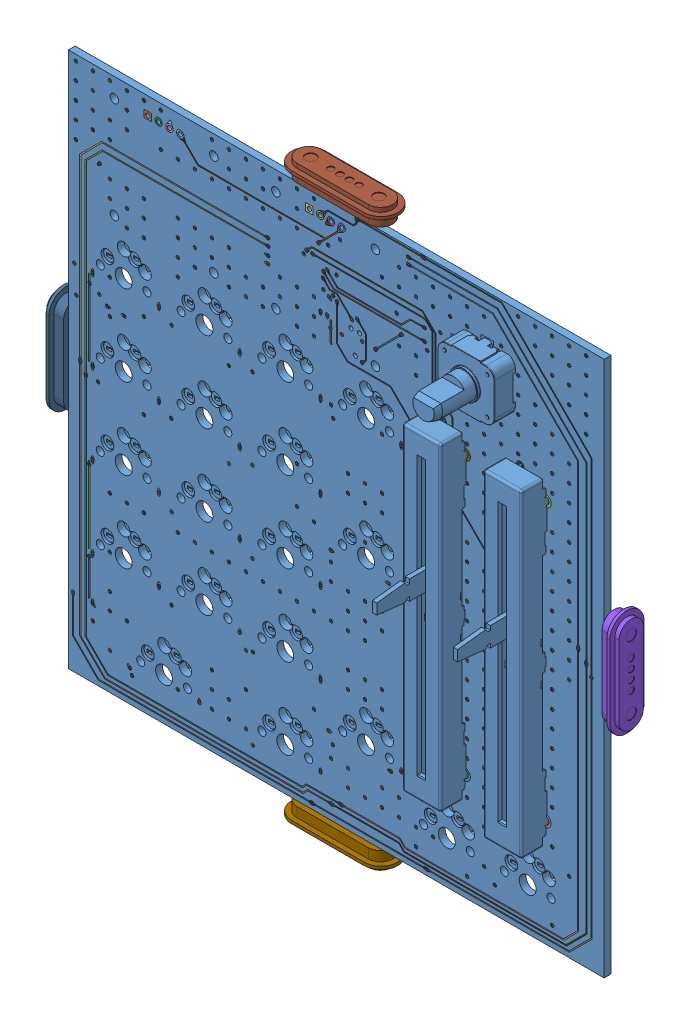
SolidWorks assembly Modulu1, configuration Default. Lengths in mm. (continued)
Components (placement in the parent): (continued)
- Numpad test 2.step-1: Numpad test 2.step [Default] at origin size (134.6 135 22.98) (continued)
  - Numpad test 2591.step-1: Numpad test 2591.step [Default] at origin size (0.81 0.81 0.01)
  - Numpad test 2592.step-1: Numpad test 2592.step [Default] at origin size (0.81 0.81 0.01)
  - Numpad test 2593.step-1: Numpad test 2593.step [Default] at origin size (0.81 0.81 0.01)
  - Numpad test 2594.step-1: Numpad test 2594.step [Default] at origin size (0.81 0.81 0.01)
  - Numpad test 2595.step-1: Numpad test 2595.step [Default] at origin size (0.81 0.81 0.01)
  - Numpad test 2596.step-1: Numpad test 2596.step [Default] at origin size (0.81 0.81 0.01)
  - Numpad test 2597.step-1: Numpad test 2597.step [Default] at origin size (0.81 0.81 0.01)
  - Numpad test 2598.step-1: Numpad test 2598.step [Default] at origin size (0.81 0.81 0.01)
  - Numpad test 2599.step-1: Numpad test 2599.step [Default] at origin size (0.81 0.81 0.01)
  - Numpad test 2600.step-1: Numpad test 2600.step [Default] at origin size (0.81 0.81 0.01)
  - Numpad test 2601.step-1: Numpad test 2601.step [Default] at origin size (0.81 0.81 0.01)
  - Numpad test 2602.step-1: Numpad test 2602.step [Default] at origin size (0.81 0.81 0.01)
  - Numpad test 2603.step-1: Numpad test 2603.step [Default] at origin size (0.81 0.81 0.01)
  - Numpad test 2604.step-1: Numpad test 2604.step [Default] at origin size (0.81 0.81 0.01)
  - Numpad test 2605.step-1: Numpad test 2605.step [Default] at origin size (0.81 0.81 0.01)
  - Numpad test 2606.step-1: Numpad test 2606.step [Default] at origin size (0.81 0.81 0.01)
  - Numpad test 2607.step-1: Numpad test 2607.step [Default] at origin size (0.81 0.81 0.01)
  - Numpad test 2608.step-1: Numpad test 2608.step [Default] at origin size (0.81 0.81 0.01)
  - Numpad test 2609.step-1: Numpad test 2609.step [Default] at origin size (0.81 0.81 0.01)
  - Numpad test 2610.step-1: Numpad test 2610.step [Default] at origin size (0.81 0.81 0.01)
  - Numpad test 2611.step-1: Numpad test 2611.step [Default] at origin size (0.81 0.81 0.01)
  - Numpad test 2612.step-1: Numpad test 2612.step [Default] at origin size (0.81 0.81 0.01)
  - Numpad test 2613.step-1: Numpad test 2613.step [Default] at origin size (0.81 0.81 0.01)
  - Numpad test 2614.step-1: Numpad test 2614.step [Default] at origin size (0.81 0.81 0.01)
  - Numpad test 2615.step-1: Numpad test 2615.step [Default] at origin size (0.81 0.81 0.01)
  - Numpad test 2616.step-1: Numpad test 2616.step [Default] at origin size (0.81 0.81 0.01)
  - Numpad test 2617.step-1: Numpad test 2617.step [Default] at origin size (0.81 0.81 0.01)
  - Numpad test 2618.step-1: Numpad test 2618.step [Default] at origin size (0.81 0.81 0.01)
  - Numpad test 2619.step-1: Numpad test 2619.step [Default] at origin size (0.81 0.81 0.01)
  - Numpad test 2620.step-1: Numpad test 2620.step [Default] at origin size (0.81 0.81 0.01)
  - Numpad test 2621.step-1: Numpad test 2621.step [Default] at origin size (0.81 0.81 0.01)
  - Numpad test 2622.step-1: Numpad test 2622.step [Default] at origin size (0.81 0.81 0.01)
  - Numpad test 2623.step-1: Numpad test 2623.step [Default] at origin size (0.81 0.81 0.01)
  - Numpad test 2624.step-1: Numpad test 2624.step [Default] at origin size (0.81 0.81 0.01)
  - Numpad test 2625.step-1: Numpad test 2625.step [Default] at origin size (0.81 0.81 0.01)
  - Numpad test 2626.step-1: Numpad test 2626.step [Default] at origin size (0.81 0.81 0.01)
  - Numpad test 2627.step-1: Numpad test 2627.step [Default] at origin size (0.81 0.81 0.01)
  - Numpad test 2628.step-1: Numpad test 2628.step [Default] at origin size (0.81 0.81 0.01)
  - Numpad test 2629.step-1: Numpad test 2629.step [Default] at origin size (0.81 0.81 0.01)
  - Numpad test 2630.step-1: Numpad test 2630.step [Default] at origin size (0.81 0.81 0.01)
  - Numpad test 2631.step-1: Numpad test 2631.step [Default] at origin size (0.81 0.81 0.01)
  - Numpad test 2632.step-1: Numpad test 2632.step [Default] at origin size (0.81 0.81 0.01)
  - Numpad test 2633.step-1: Numpad test 2633.step [Default] at origin size (0.81 0.81 0.01)
  - Numpad test 2634.step-1: Numpad test 2634.step [Default] at origin size (0.81 0.81 0.01)
  - Numpad test 2635.step-1: Numpad test 2635.step [Default] at origin size (0.81 0.81 0.01)
  - Numpad test 2636.step-1: Numpad test 2636.step [Default] at origin size (0.81 0.81 0.01)
  - Numpad test 2637.step-1: Numpad test 2637.step [Default] at origin size (0.81 0.81 0.01)
  - Numpad test 2638.step-1: Numpad test 2638.step [Default] at origin size (0.81 0.81 0.01)
  - Numpad test 2639.step-1: Numpad test 2639.step [Default] at origin size (0.81 0.81 0.01)
  - Numpad test 2640.step-1: Numpad test 2640.step [Default] at origin size (0.81 0.81 0.01)
  - Numpad test 2641.step-1: Numpad test 2641.step [Default] at origin size (0.81 0.81 0.01)
  - Numpad test 2642.step-1: Numpad test 2642.step [Default] at origin size (0.81 0.81 0.01)
  - Numpad test 2643.step-1: Numpad test 2643.step [Default] at origin size (0.81 0.81 0.01)
  - Numpad test 2644.step-1: Numpad test 2644.step [Default] at origin size (0.81 0.81 0.01)
  - Numpad test 2645.step-1: Numpad test 2645.step [Default] at origin size (0.81 0.81 0.01)
  - Numpad test 2646.step-1: Numpad test 2646.step [Default] at origin size (0.81 0.81 0.01)
  - Numpad test 2647.step-1: Numpad test 2647.step [Default] at origin size (0.81 0.81 0.01)
  - Numpad test 2648.step-1: Numpad test 2648.step [Default] at origin size (0.81 0.81 0.01)
  - Numpad test 2649.step-1: Numpad test 2649.step [Default] at origin size (0.81 0.81 0.01)
  - Numpad test 2650.step-1: Numpad test 2650.step [Default] at origin size (0.81 0.81 0.01)
  - Numpad test 2651.step-1: Numpad test 2651.step [Default] at origin size (0.81 0.81 0.01)
  - Numpad test 2652.step-1: Numpad test 2652.step [Default] at origin size (0.81 0.81 0.01)
  - Numpad test 2653.step-1: Numpad test 2653.step [Default] at origin size (0.81 0.81 0.01)
  - Numpad test 2654.step-1: Numpad test 2654.step [Default] at origin size (0.81 0.81 0.01)
  - Numpad test 2655.step-1: Numpad test 2655.step [Default] at origin size (0.81 0.81 0.01)
  - Numpad test 2656.step-1: Numpad test 2656.step [Default] at origin size (0.81 0.81 0.01)
  - Numpad test 2657.step-1: Numpad test 2657.step [Default] at origin size (0.81 0.81 0.01)
  - Numpad test 2658.step-1: Numpad test 2658.step [Default] at origin size (0.81 0.81 0.01)
  - Numpad test 2659.step-1: Numpad test 2659.step [Default] at origin size (0.81 0.81 0.01)
  - Numpad test 2660.step-1: Numpad test 2660.step [Default] at origin size (0.81 0.81 0.01)
  - Numpad test 2661.step-1: Numpad test 2661.step [Default] at origin size (0.81 0.81 0.01)
  - Numpad test 2662.step-1: Numpad test 2662.step [Default] at origin size (0.81 0.81 0.01)
  - Numpad test 2663.step-1: Numpad test 2663.step [Default] at origin size (0.81 0.81 0.01)
  - Numpad test 2664.step-1: Numpad test 2664.step [Default] at origin size (0.81 0.81 0.01)
  - Numpad test 2665.step-1: Numpad test 2665.step [Default] at origin size (0.81 0.81 0.01)
  - Numpad test 2666.step-1: Numpad test 2666.step [Default] at origin size (0.81 0.81 0.01)
  - Numpad test 2667.step-1: Numpad test 2667.step [Default] at origin size (0.81 0.81 0.01)
  - Numpad test 2668.step-1: Numpad test 2668.step [Default] at origin size (0.81 0.81 0.01)
  - Numpad test 2669.step-1: Numpad test 2669.step [Default] at origin size (0.81 0.81 0.01)
  - Numpad test 2670.step-1: Numpad test 2670.step [Default] at origin size (0.81 0.81 0.01)
  - Numpad test 2671.step-1: Numpad test 2671.step [Default] at origin size (0.81 0.81 0.01)
  - Numpad test 2672.step-1: Numpad test 2672.step [Default] at origin size (0.81 0.81 0.01)
  - Numpad test 2673.step-1: Numpad test 2673.step [Default] at origin size (0.81 0.81 0.01)
  - Numpad test 2674.step-1: Numpad test 2674.step [Default] at origin size (0.81 0.81 0.01)
  - Numpad test 2675.step-1: Numpad test 2675.step [Default] at origin size (0.81 0.81 0.01)
  - Numpad test 2676.step-1: Numpad test 2676.step [Default] at origin size (0.81 0.81 0.01)
  - Numpad test 2677.step-1: Numpad test 2677.step [Default] at origin size (0.81 0.81 0.01)
  - Numpad test 2678.step-1: Numpad test 2678.step [Default] at origin size (0.81 0.81 0.01)
  - Numpad test 2679.step-1: Numpad test 2679.step [Default] at origin size (0.81 0.81 0.01)
  - Numpad test 2680.step-1: Numpad test 2680.step [Default] at origin size (0.81 0.81 0.01)
  - Numpad test 2681.step-1: Numpad test 2681.step [Default] at origin size (0.81 0.81 0.01)
  - Numpad test 2682.step-1: Numpad test 2682.step [Default] at origin size (0.81 0.81 0.01)
  - Numpad test 2683.step-1: Numpad test 2683.step [Default] at origin size (4.61 4.61 0.01)
  - Numpad test 2684.step-1: Numpad test 2684.step [Default] at origin size (4.61 4.61 0.01)
  - Numpad test 2685.step-1: Numpad test 2685.step [Default] at origin size (4.57 3.92 0.01)
  - Numpad test 2686.step-1: Numpad test 2686.step [Default] at origin size (4.57 3.92 0.01)
  - Numpad test 2687.step-1: Numpad test 2687.step [Default] at origin size (4.57 3.92 0.01)
  - Numpad test 2688.step-1: Numpad test 2688.step [Default] at origin size (4.57 3.92 0.01)
  - Numpad test 2689.step-1: Numpad test 2689.step [Default] at origin size (4.57 3.92 0.01)
  - Numpad test 2690.step-1: Numpad test 2690.step [Default] at origin size (4.57 3.92 0.01)
  - Numpad test 2691.step-1: Numpad test 2691.step [Default] at origin size (4.57 3.92 0.01)
  - Numpad test 2692.step-1: Numpad test 2692.step [Default] at origin size (4.57 3.92 0.01)
  - Numpad test 2693.step-1: Numpad test 2693.step [Default] at origin size (4.57 3.92 0.01)
  - Numpad test 2694.step-1: Numpad test 2694.step [Default] at origin size (4.57 3.92 0.01)
  - Numpad test 2695.step-1: Numpad test 2695.step [Default] at origin size (4.57 3.92 0.01)
  - Numpad test 2696.step-1: Numpad test 2696.step [Default] at origin size (4.57 3.92 0.01)
  - Numpad test 2697.step-1: Numpad test 2697.step [Default] at origin size (4.57 3.92 0.01)
  - Numpad test 2698.step-1: Numpad test 2698.step [Default] at origin size (4.57 3.92 0.01)
  - Numpad test 2699.step-1: Numpad test 2699.step [Default] at origin size (4.57 3.92 0.01)
  - Numpad test 2700.step-1: Numpad test 2700.step [Default] at origin size (4.57 3.92 0.01)
  - Numpad test 2701.step-1: Numpad test 2701.step [Default] at origin size (4.57 3.92 0.01)
  - Numpad test 2702.step-1: Numpad test 2702.step [Default] at origin size (4.57 3.92 0.01)
  - Numpad test 2703.step-1: Numpad test 2703.step [Default] at origin size (4.57 3.92 0.01)
  - Numpad test 2704.step-1: Numpad test 2704.step [Default] at origin size (3.01 2.51 0.01)
  - Numpad test 2705.step-1: Numpad test 2705.step [Default] at origin size (3.01 2.51 0.01)
  - Numpad test 2706.step-1: Numpad test 2706.step [Default] at origin size (2.71 2.71 0.01)
  - Numpad test 2707.step-1: Numpad test 2707.step [Default] at origin size (2.71 2.71 0.01)
  - Numpad test 2708.step-1: Numpad test 2708.step [Default] at origin size (2.71 2.71 0.01)
  - Numpad test 2709.step-1: Numpad test 2709.step [Default] at origin size (2.71 2.71 0.01)
  - Numpad test 2710.step-1: Numpad test 2710.step [Default] at origin size (2.71 2.71 0.01)
  - Numpad test 2711.step-1: Numpad test 2711.step [Default] at origin size (2.71 2.71 0.01)
  - Numpad test 2712.step-1: Numpad test 2712.step [Default] at origin size (2.71 2.71 0.01)
  - Numpad test 2713.step-1: Numpad test 2713.step [Default] at origin size (2.71 2.71 0.01)
  - Numpad test 2714.step-1: Numpad test 2714.step [Default] at origin size (2.61 2.61 0.01)
  - Numpad test 2715.step-1: Numpad test 2715.step [Default] at origin size (2.61 2.61 0.01)
  - Numpad test 2716.step-1: Numpad test 2716.step [Default] at origin size (2.61 2.61 0.01)
  - Numpad test 2717.step-1: Numpad test 2717.step [Default] at origin size (2.61 2.61 0.01)
  - Numpad test 2718.step-1: Numpad test 2718.step [Default] at origin size (2.61 2.61 0.01)
  - Numpad test 2719.step-1: Numpad test 2719.step [Default] at origin size (2.61 2.61 0.01)
  - Numpad test 2720.step-1: Numpad test 2720.step [Default] at origin size (2.61 2.61 0.01)
  - Numpad test 2721.step-1: Numpad test 2721.step [Default] at origin size (2.61 2.61 0.01)
  - Numpad test 2722.step-1: Numpad test 2722.step [Default] at origin size (2.61 2.61 0.01)
  - Numpad test 2723.step-1: Numpad test 2723.step [Default] at origin size (2.61 2.61 0.01)
  - Numpad test 2724.step-1: Numpad test 2724.step [Default] at origin size (2.61 2.61 0.01)
  - Numpad test 2725.step-1: Numpad test 2725.step [Default] at origin size (2.61 2.61 0.01)
  - Numpad test 2726.step-1: Numpad test 2726.step [Default] at origin size (2.61 2.61 0.01)
  - Numpad test 2727.step-1: Numpad test 2727.step [Default] at origin size (2.61 2.61 0.01)
  - Numpad test 2728.step-1: Numpad test 2728.step [Default] at origin size (2.61 2.61 0.01)
  - Numpad test 2729.step-1: Numpad test 2729.step [Default] at origin size (2.61 2.61 0.01)
  - Numpad test 2730.step-1: Numpad test 2730.step [Default] at origin size (2.61 2.61 0.01)
  - Numpad test 2731.step-1: Numpad test 2731.step [Default] at origin size (2.61 2.61 0.01)
  - Numpad test 2732.step-1: Numpad test 2732.step [Default] at origin size (2.61 2.61 0.01)
  - Numpad test 2733.step-1: Numpad test 2733.step [Default] at origin size (2.55 2.55 0.01)
  - Numpad test 2734.step-1: Numpad test 2734.step [Default] at origin size (2.55 2.55 0.01)
  - Numpad test 2735.step-1: Numpad test 2735.step [Default] at origin size (2.55 2.55 0.01)
  - Numpad test 2736.step-1: Numpad test 2736.step [Default] at origin size (2.55 2.55 0.01)
  - Numpad test 2737.step-1: Numpad test 2737.step [Default] at origin size (2.55 2.55 0.01)
  - Numpad test 2738.step-1: Numpad test 2738.step [Default] at origin size (2.55 2.55 0.01)
  - Numpad test 2739.step-1: Numpad test 2739.step [Default] at origin size (2.55 2.55 0.01)
  - Numpad test 2740.step-1: Numpad test 2740.step [Default] at origin size (2.55 2.55 0.01)
  - Numpad test 2741.step-1: Numpad test 2741.step [Default] at origin size (2.55 2.55 0.01)
  - Numpad test 2742.step-1: Numpad test 2742.step [Default] at origin size (2.55 2.55 0.01)
  - Numpad test 2743.step-1: Numpad test 2743.step [Default] at origin size (2.55 2.55 0.01)
  - Numpad test 2744.step-1: Numpad test 2744.step [Default] at origin size (2.55 2.55 0.01)
  - Numpad test 2745.step-1: Numpad test 2745.step [Default] at origin size (2.55 2.55 0.01)
  - Numpad test 2746.step-1: Numpad test 2746.step [Default] at origin size (2.55 2.55 0.01)
  - Numpad test 2747.step-1: Numpad test 2747.step [Default] at origin size (2.55 2.55 0.01)
  - Numpad test 2748.step-1: Numpad test 2748.step [Default] at origin size (2.55 2.55 0.01)
  - Numpad test 2749.step-1: Numpad test 2749.step [Default] at origin size (2.55 2.55 0.01)
  - Numpad test 2750.step-1: Numpad test 2750.step [Default] at origin size (2.55 2.55 0.01)
  - Numpad test 2751.step-1: Numpad test 2751.step [Default] at origin size (2.55 2.55 0.01)
  - Numpad test 2752.step-1: Numpad test 2752.step [Default] at origin size (2.01 2.01 0.01)
  - Numpad test 2753.step-1: Numpad test 2753.step [Default] at origin size (2.01 2.01 0.01)
  - Numpad test 2754.step-1: Numpad test 2754.step [Default] at origin size (2.01 2.01 0.01)
  - Numpad test 2755.step-1: Numpad test 2755.step [Default] at origin size (0.81 2.06 0.01)
  - Numpad test 2756.step-1: Numpad test 2756.step [Default] at origin size (2.06 0.81 0.01)
  - Numpad test 2757.step-1: Numpad test 2757.step [Default] at origin size (2.06 0.81 0.01)
  - Numpad test 2758.step-1: Numpad test 2758.step [Default] at origin size (0.81 2.06 0.01)
  - Numpad test 2759.step-1: Numpad test 2759.step [Default] at origin size (2.16 0.81 0.01)
  - Numpad test 2760.step-1: Numpad test 2760.step [Default] at origin size (0.81 1.76 0.01)
  - Numpad test 2761.step-1: Numpad test 2761.step [Default] at origin size (0.81 1.76 0.01)
  - Numpad test 2762.step-1: Numpad test 2762.step [Default] at origin size (2.16 0.81 0.01)
  - Numpad test 2763.step-1: Numpad test 2763.step [Default] at origin size (2.06 0.81 0.01)
  - Numpad test 2764.step-1: Numpad test 2764.step [Default] at origin size (2.06 0.81 0.01)
  - Numpad test 2765.step-1: Numpad test 2765.step [Default] at origin size (0.81 2.06 0.01)
  - Numpad test 2766.step-1: Numpad test 2766.step [Default] at origin size (0.81 1.76 0.01)
  - Numpad test 2767.step-1: Numpad test 2767.step [Default] at origin size (0.81 2.06 0.01)
  - Numpad test 2768.step-1: Numpad test 2768.step [Default] at origin size (0.81 1.76 0.01)
  - Numpad test 2769.step-1: Numpad test 2769.step [Default] at origin size (2.16 0.81 0.01)
  - Numpad test 2770.step-1: Numpad test 2770.step [Default] at origin size (2.16 0.81 0.01)
  - Numpad test 2771.step-1: Numpad test 2771.step [Default] at origin size (1.76 1.76 0.01)
  - Numpad test 2772.step-1: Numpad test 2772.step [Default] at origin size (1.76 1.76 0.01)
  - Numpad test 2773.step-1: Numpad test 2773.step [Default] at origin size (1.76 1.76 0.01)
  - Numpad test 2774.step-1: Numpad test 2774.step [Default] at origin size (1.76 1.76 0.01)
  - Numpad test 2775.step-1: Numpad test 2775.step [Default] at origin size (1.76 1.76 0.01)
  - Numpad test 2776.step-1: Numpad test 2776.step [Default] at origin size (1.76 1.76 0.01)
  - Numpad test 2777.step-1: Numpad test 2777.step [Default] at origin size (1.71 1.71 0.01)
  - Numpad test 2778.step-1: Numpad test 2778.step [Default] at origin size (1.71 1.71 0.01)
  - Numpad test 2779.step-1: Numpad test 2779.step [Default] at origin size (1.71 1.71 0.01)
  - Numpad test 2780.step-1: Numpad test 2780.step [Default] at origin size (1.71 1.71 0.01)
  - Numpad test 2781.step-1: Numpad test 2781.step [Default] at origin size (1.71 1.71 0.01)
  - Numpad test 2782.step-1: Numpad test 2782.step [Default] at origin size (1.71 1.71 0.01)
  - Numpad test 2783.step-1: Numpad test 2783.step [Default] at origin size (1.71 1.71 0.01)
  - Numpad test 2784.step-1: Numpad test 2784.step [Default] at origin size (1.71 1.71 0.01)
  - Numpad test 2785.step-1: Numpad test 2785.step [Default] at origin size (1.91 0.83 0.01)
  - Numpad test 2786.step-1: Numpad test 2786.step [Default] at origin size (1.91 0.83 0.01)
  - Numpad test 2787.step-1: Numpad test 2787.step [Default] at origin size (1.91 0.83 0.01)
  - Numpad test 2788.step-1: Numpad test 2788.step [Default] at origin size (1.91 0.83 0.01)
  - Numpad test 2789.step-1: Numpad test 2789.step [Default] at origin size (1.91 0.83 0.01)
  - Numpad test 2790.step-1: Numpad test 2790.step [Default] at origin size (1.91 0.83 0.01)
  - Numpad test 2791.step-1: Numpad test 2791.step [Default] at origin size (1.91 0.83 0.01)
  - Numpad test 2792.step-1: Numpad test 2792.step [Default] at origin size (1.91 0.83 0.01)
  - Numpad test 2793.step-1: Numpad test 2793.step [Default] at origin size (1.91 0.83 0.01)
  - Numpad test 2794.step-1: Numpad test 2794.step [Default] at origin size (1.91 0.83 0.01)
  - Numpad test 2795.step-1: Numpad test 2795.step [Default] at origin size (1.91 0.83 0.01)
  - Numpad test 2796.step-1: Numpad test 2796.step [Default] at origin size (1.91 0.83 0.01)
  - Numpad test 2797.step-1: Numpad test 2797.step [Default] at origin size (1.91 0.83 0.01)
  - Numpad test 2798.step-1: Numpad test 2798.step [Default] at origin size (1.91 0.83 0.01)
  - Numpad test 2799.step-1: Numpad test 2799.step [Default] at origin size (1.91 0.83 0.01)
  - Numpad test 2800.step-1: Numpad test 2800.step [Default] at origin size (1.91 0.83 0.01)
  - Numpad test 2801.step-1: Numpad test 2801.step [Default] at origin size (1.91 0.83 0.01)
  - Numpad test 2802.step-1: Numpad test 2802.step [Default] at origin size (1.91 0.83 0.01)
  - Numpad test 2803.step-1: Numpad test 2803.step [Default] at origin size (1.91 0.83 0.01)
  - Numpad test 2804.step-1: Numpad test 2804.step [Default] at origin size (1.91 0.83 0.01)
  - Numpad test 2805.step-1: Numpad test 2805.step [Default] at origin size (1.91 0.83 0.01)
  - Numpad test 2806.step-1: Numpad test 2806.step [Default] at origin size (1.91 0.83 0.01)
  - Numpad test 2807.step-1: Numpad test 2807.step [Default] at origin size (1.91 0.83 0.01)
  - Numpad test 2808.step-1: Numpad test 2808.step [Default] at origin size (1.91 0.83 0.01)
  - Numpad test 2809.step-1: Numpad test 2809.step [Default] at origin size (1.91 0.83 0.01)
  - Numpad test 2810.step-1: Numpad test 2810.step [Default] at origin size (1.91 0.83 0.01)
  - Numpad test 2811.step-1: Numpad test 2811.step [Default] at origin size (1.91 0.83 0.01)
  - Numpad test 2812.step-1: Numpad test 2812.step [Default] at origin size (1.91 0.83 0.01)
  - Numpad test 2813.step-1: Numpad test 2813.step [Default] at origin size (1.91 0.83 0.01)
  - Numpad test 2814.step-1: Numpad test 2814.step [Default] at origin size (1.91 0.83 0.01)
  - Numpad test 2815.step-1: Numpad test 2815.step [Default] at origin size (1.91 0.83 0.01)
  - Numpad test 2816.step-1: Numpad test 2816.step [Default] at origin size (1.91 0.83 0.01)
  - Numpad test 2817.step-1: Numpad test 2817.step [Default] at origin size (1.91 0.83 0.01)
  - Numpad test 2818.step-1: Numpad test 2818.step [Default] at origin size (1.91 0.83 0.01)
  - Numpad test 2819.step-1: Numpad test 2819.step [Default] at origin size (1.91 0.83 0.01)
  - Numpad test 2820.step-1: Numpad test 2820.step [Default] at origin size (1.91 0.83 0.01)
  - Numpad test 2821.step-1: Numpad test 2821.step [Default] at origin size (1.91 0.83 0.01)
  - Numpad test 2822.step-1: Numpad test 2822.step [Default] at origin size (1.91 0.83 0.01)
  - Numpad test 2823.step-1: Numpad test 2823.step [Default] at origin size (1.91 0.83 0.01)
  - Numpad test 2824.step-1: Numpad test 2824.step [Default] at origin size (1.91 0.83 0.01)
  - Numpad test 2825.step-1: Numpad test 2825.step [Default] at origin size (1.91 0.83 0.01)
  - Numpad test 2826.step-1: Numpad test 2826.step [Default] at origin size (1.91 0.83 0.01)
  - Numpad test 2827.step-1: Numpad test 2827.step [Default] at origin size (1.91 0.83 0.01)
  - Numpad test 2828.step-1: Numpad test 2828.step [Default] at origin size (1.91 0.83 0.01)
  - Numpad test 2829.step-1: Numpad test 2829.step [Default] at origin size (1.91 0.83 0.01)
  - Numpad test 2830.step-1: Numpad test 2830.step [Default] at origin size (1.91 0.83 0.01)
  - Numpad test 2831.step-1: Numpad test 2831.step [Default] at origin size (1.91 0.83 0.01)
  - Numpad test 2832.step-1: Numpad test 2832.step [Default] at origin size (1.91 0.83 0.01)
  - Numpad test 2833.step-1: Numpad test 2833.step [Default] at origin size (1.91 0.83 0.01)
  - Numpad test 2834.step-1: Numpad test 2834.step [Default] at origin size (1.91 0.83 0.01)
  - Numpad test 2835.step-1: Numpad test 2835.step [Default] at origin size (1.91 0.83 0.01)
  - Numpad test 2836.step-1: Numpad test 2836.step [Default] at origin size (1.91 0.83 0.01)
  - Numpad test 2837.step-1: Numpad test 2837.step [Default] at origin size (1.91 0.83 0.01)
  - Numpad test 2838.step-1: Numpad test 2838.step [Default] at origin size (1.91 0.83 0.01)
  - Numpad test 2839.step-1: Numpad test 2839.step [Default] at origin size (1.91 0.83 0.01)
  - Numpad test 2840.step-1: Numpad test 2840.step [Default] at origin size (1.91 0.83 0.01)
  - Numpad test 2841.step-1: Numpad test 2841.step [Default] at origin size (1.91 0.83 0.01)
  - Numpad test 2842.step-1: Numpad test 2842.step [Default] at origin size (1.91 0.83 0.01)
  - Numpad test 2843.step-1: Numpad test 2843.step [Default] at origin size (1.91 0.83 0.01)
  - Numpad test 2844.step-1: Numpad test 2844.step [Default] at origin size (1.91 0.83 0.01)
  - Numpad test 2845.step-1: Numpad test 2845.step [Default] at origin size (1.91 0.83 0.01)
  - Numpad test 2846.step-1: Numpad test 2846.step [Default] at origin size (1.91 0.83 0.01)
  - Numpad test 2847.step-1: Numpad test 2847.step [Default] at origin size (1.91 0.83 0.01)
  - Numpad test 2848.step-1: Numpad test 2848.step [Default] at origin size (1.91 0.83 0.01)
  - Numpad test 2849.step-1: Numpad test 2849.step [Default] at origin size (1.91 0.83 0.01)
  - Numpad test 2850.step-1: Numpad test 2850.step [Default] at origin size (1.91 0.83 0.01)
  - Numpad test 2851.step-1: Numpad test 2851.step [Default] at origin size (1.91 0.83 0.01)
  - Numpad test 2852.step-1: Numpad test 2852.step [Default] at origin size (1.91 0.83 0.01)
  - Numpad test 2853.step-1: Numpad test 2853.step [Default] at origin size (1.91 0.83 0.01)
  - Numpad test 2854.step-1: Numpad test 2854.step [Default] at origin size (1.91 0.83 0.01)
  - Numpad test 2855.step-1: Numpad test 2855.step [Default] at origin size (1.91 0.83 0.01)
  - Numpad test 2856.step-1: Numpad test 2856.step [Default] at origin size (1.91 0.83 0.01)
  - Numpad test 2857.step-1: Numpad test 2857.step [Default] at origin size (1.91 0.83 0.01)
  - Numpad test 2858.step-1: Numpad test 2858.step [Default] at origin size (1.91 0.83 0.01)
  - Numpad test 2859.step-1: Numpad test 2859.step [Default] at origin size (1.91 0.83 0.01)
  - Numpad test 2860.step-1: Numpad test 2860.step [Default] at origin size (1.91 0.83 0.01)
  - Numpad test 2861.step-1: Numpad test 2861.step [Default] at origin size (1.91 0.83 0.01)
  - Numpad test 2862.step-1: Numpad test 2862.step [Default] at origin size (1.91 0.83 0.01)
  - Numpad test 2863.step-1: Numpad test 2863.step [Default] at origin size (1.91 0.83 0.01)
  - Numpad test 2864.step-1: Numpad test 2864.step [Default] at origin size (1.91 0.83 0.01)
  - Numpad test 2865.step-1: Numpad test 2865.step [Default] at origin size (0.56 1.61 0.01)
  - Numpad test 2866.step-1: Numpad test 2866.step [Default] at origin size (0.56 1.61 0.01)
  - Numpad test 2867.step-1: Numpad test 2867.step [Default] at origin size (0.56 1.61 0.01)
  - Numpad test 2868.step-1: Numpad test 2868.step [Default] at origin size (0.56 1.61 0.01)
  - Numpad test 2869.step-1: Numpad test 2869.step [Default] at origin size (0.56 1.61 0.01)
  - Numpad test 2870.step-1: Numpad test 2870.step [Default] at origin size (1.61 0.56 0.01)
  - Numpad test 2871.step-1: Numpad test 2871.step [Default] at origin size (1.61 0.56 0.01)
  - Numpad test 2872.step-1: Numpad test 2872.step [Default] at origin size (1.61 0.56 0.01)
  - Numpad test 2873.step-1: Numpad test 2873.step [Default] at origin size (1.61 0.56 0.01)
  - Numpad test 2874.step-1: Numpad test 2874.step [Default] at origin size (1.61 0.56 0.01)
  - Numpad test 2875.step-1: Numpad test 2875.step [Default] at origin size (1.61 0.56 0.01)
  - Numpad test 2876.step-1: Numpad test 2876.step [Default] at origin size (1.61 0.56 0.01)
  - Numpad test 2877.step-1: Numpad test 2877.step [Default] at origin size (1.61 0.56 0.01)
  - Numpad test 2878.step-1: Numpad test 2878.step [Default] at origin size (1.61 0.56 0.01)
  - Numpad test 2879.step-1: Numpad test 2879.step [Default] at origin size (1.61 0.56 0.01)
  - Numpad test 2880.step-1: Numpad test 2880.step [Default] at origin size (1.61 0.56 0.01)
  - Numpad test 2881.step-1: Numpad test 2881.step [Default] at origin size (1.61 0.56 0.01)
  - Numpad test 2882.step-1: Numpad test 2882.step [Default] at origin size (1.61 0.56 0.01)
  - Numpad test 2883.step-1: Numpad test 2883.step [Default] at origin size (1.61 0.56 0.01)
  - Numpad test 2884.step-1: Numpad test 2884.step [Default] at origin size (1.61 0.56 0.01)
  - Numpad test 2885.step-1: Numpad test 2885.step [Default] at origin size (1.61 0.56 0.01)
  - Numpad test 2886.step-1: Numpad test 2886.step [Default] at origin size (0.56 1.61 0.01)
  - Numpad test 2887.step-1: Numpad test 2887.step [Default] at origin size (0.56 1.61 0.01)
  - Numpad test 2888.step-1: Numpad test 2888.step [Default] at origin size (0.56 1.61 0.01)
  - Numpad test 2889.step-1: Numpad test 2889.step [Default] at origin size (0.56 1.61 0.01)
  - Numpad test 2890.step-1: Numpad test 2890.step [Default] at origin size (0.56 1.61 0.01)
  - Numpad test 2891.step-1: Numpad test 2891.step [Default] at origin size (0.56 1.61 0.01)
  - Numpad test 2892.step-1: Numpad test 2892.step [Default] at origin size (0.56 1.61 0.01)
  - Numpad test 2893.step-1: Numpad test 2893.step [Default] at origin size (0.56 1.61 0.01)
  - Numpad test 2894.step-1: Numpad test 2894.step [Default] at origin size (0.56 1.61 0.01)
  - Numpad test 2895.step-1: Numpad test 2895.step [Default] at origin size (0.56 1.61 0.01)
  - Numpad test 2896.step-1: Numpad test 2896.step [Default] at origin size (0.56 1.61 0.01)
  - Numpad test 2897.step-1: Numpad test 2897.step [Default] at origin size (1.13 1.13 0.01)
  - Numpad test 2898.step-1: Numpad test 2898.step [Default] at origin size (1.13 1.13 0.01)
  - Numpad test 2899.step-1: Numpad test 2899.step [Default] at origin size (1.13 1.13 0.01)
  - Numpad test 2900.step-1: Numpad test 2900.step [Default] at origin size (1.13 1.13 0.01)
  - Numpad test 2901.step-1: Numpad test 2901.step [Default] at origin size (0.91 0.96 0.01)
  - Numpad test 2902.step-1: Numpad test 2902.step [Default] at origin size (0.91 0.96 0.01)
  - Numpad test 2903.step-1: Numpad test 2903.step [Default] at origin size (0.91 0.96 0.01)
  - Numpad test 2904.step-1: Numpad test 2904.step [Default] at origin size (0.91 0.96 0.01)
  - Numpad test 2905.step-1: Numpad test 2905.step [Default] at origin size (0.91 0.96 0.01)
  - Numpad test 2906.step-1: Numpad test 2906.step [Default] at origin size (0.91 0.96 0.01)
  - Numpad test 2907.step-1: Numpad test 2907.step [Default] at origin size (0.96 0.91 0.01)
  - Numpad test 2908.step-1: Numpad test 2908.step [Default] at origin size (0.91 0.96 0.01)
  - Numpad test 2909.step-1: Numpad test 2909.step [Default] at origin size (0.91 0.96 0.01)
  - Numpad test 2910.step-1: Numpad test 2910.step [Default] at origin size (0.96 0.91 0.01)
  - Numpad test 2911.step-1: Numpad test 2911.step [Default] at origin size (0.96 0.91 0.01)
  - Numpad test 2912.step-1: Numpad test 2912.step [Default] at origin size (0.91 0.96 0.01)
  - Numpad test 2913.step-1: Numpad test 2913.step [Default] at origin size (0.91 0.96 0.01)
  - Numpad test 2914.step-1: Numpad test 2914.step [Default] at origin size (0.91 0.96 0.01)
  - Numpad test 2915.step-1: Numpad test 2915.step [Default] at origin size (0.91 0.96 0.01)
  - Numpad test 2916.step-1: Numpad test 2916.step [Default] at origin size (0.91 0.96 0.01)
  - Numpad test 2917.step-1: Numpad test 2917.step [Default] at origin size (0.91 0.96 0.01)
  - Numpad test 2918.step-1: Numpad test 2918.step [Default] at origin size (0.91 0.96 0.01)
  - Numpad test 2919.step-1: Numpad test 2919.step [Default] at origin size (0.96 0.91 0.01)
  - Numpad test 2920.step-1: Numpad test 2920.step [Default] at origin size (0.91 0.96 0.01)
  - Numpad test 2921.step-1: Numpad test 2921.step [Default] at origin size (0.96 0.91 0.01)
  - Numpad test 2922.step-1: Numpad test 2922.step [Default] at origin size (0.91 0.96 0.01)
  - Numpad test 2923.step-1: Numpad test 2923.step [Default] at origin size (0.96 0.91 0.01)
  - Numpad test 2924.step-1: Numpad test 2924.step [Default] at origin size (0.91 0.96 0.01)
  - Numpad test 2925.step-1: Numpad test 2925.step [Default] at origin size (0.91 0.96 0.01)
  - Numpad test 2926.step-1: Numpad test 2926.step [Default] at origin size (0.91 0.96 0.01)
  - Numpad test 2927.step-1: Numpad test 2927.step [Default] at origin size (0.91 0.96 0.01)
  - Numpad test 2928.step-1: Numpad test 2928.step [Default] at origin size (0.91 0.96 0.01)
  - Numpad test 2929.step-1: Numpad test 2929.step [Default] at origin size (0.91 0.96 0.01)
  - Numpad test 2930.step-1: Numpad test 2930.step [Default] at origin size (0.91 0.96 0.01)
  - Numpad test 2931.step-1: Numpad test 2931.step [Default] at origin size (0.91 0.96 0.01)
  - Numpad test 2932.step-1: Numpad test 2932.step [Default] at origin size (0.91 0.96 0.01)
  - Numpad test 2933.step-1: Numpad test 2933.step [Default] at origin size (0.91 0.96 0.01)
  - Numpad test 2934.step-1: Numpad test 2934.step [Default] at origin size (0.91 0.96 0.01)
  - Numpad test 2935.step-1: Numpad test 2935.step [Default] at origin size (0.91 0.96 0.01)
  - Numpad test 2936.step-1: Numpad test 2936.step [Default] at origin size (0.91 0.96 0.01)
  - Numpad test 2937.step-1: Numpad test 2937.step [Default] at origin size (0.91 0.96 0.01)
  - Numpad test 2938.step-1: Numpad test 2938.step [Default] at origin size (0.91 0.96 0.01)
  - Numpad test 2939.step-1: Numpad test 2939.step [Default] at origin size (0.91 0.96 0.01)
  - Numpad test 2940.step-1: Numpad test 2940.step [Default] at origin size (0.91 0.96 0.01)
  - Numpad test 2941.step-1: Numpad test 2941.step [Default] at origin size (0.91 0.96 0.01)
  - Numpad test 2942.step-1: Numpad test 2942.step [Default] at origin size (0.91 0.96 0.01)
  - Numpad test 2943.step-1: Numpad test 2943.step [Default] at origin size (0.91 0.96 0.01)
  - Numpad test 2944.step-1: Numpad test 2944.step [Default] at origin size (0.91 0.96 0.01)
  - Numpad test 2945.step-1: Numpad test 2945.step [Default] at origin size (0.91 0.96 0.01)
  - Numpad test 2946.step-1: Numpad test 2946.step [Default] at origin size (0.91 0.96 0.01)
  - Numpad test 2947.step-1: Numpad test 2947.step [Default] at origin size (0.91 0.96 0.01)
  - Numpad test 2948.step-1: Numpad test 2948.step [Default] at origin size (0.91 0.96 0.01)
  - Numpad test 2949.step-1: Numpad test 2949.step [Default] at origin size (0.96 0.91 0.01)
  - Numpad test 2950.step-1: Numpad test 2950.step [Default] at origin size (0.91 0.96 0.01)
  - Numpad test 2951.step-1: Numpad test 2951.step [Default] at origin size (0.96 0.91 0.01)
  - Numpad test 2952.step-1: Numpad test 2952.step [Default] at origin size (0.96 0.91 0.01)
  - Numpad test 2953.step-1: Numpad test 2953.step [Default] at origin size (0.96 0.91 0.01)
  - Numpad test 2954.step-1: Numpad test 2954.step [Default] at origin size (0.91 0.96 0.01)
  - Numpad test 2955.step-1: Numpad test 2955.step [Default] at origin size (0.96 0.89 0.01)
  - Numpad test 2956.step-1: Numpad test 2956.step [Default] at origin size (0.96 0.89 0.01)
  - Numpad test 2957.step-1: Numpad test 2957.step [Default] at origin size (0.96 0.89 0.01)
  - Numpad test 2958.step-1: Numpad test 2958.step [Default] at origin size (0.96 0.89 0.01)
  - Numpad test 2959.step-1: Numpad test 2959.step [Default] at origin size (0.96 0.89 0.01)
  - Numpad test 2960.step-1: Numpad test 2960.step [Default] at origin size (0.96 0.89 0.01)
  - Numpad test 2961.step-1: Numpad test 2961.step [Default] at origin size (0.96 0.89 0.01)
  - Numpad test 2962.step-1: Numpad test 2962.step [Default] at origin size (0.96 0.89 0.01)
  - Numpad test 2963.step-1: Numpad test 2963.step [Default] at origin size (0.96 0.89 0.01)
  - Numpad test 2964.step-1: Numpad test 2964.step [Default] at origin size (0.96 0.89 0.01)
  - Numpad test 2965.step-1: Numpad test 2965.step [Default] at origin size (0.96 0.89 0.01)
  - Numpad test 2966.step-1: Numpad test 2966.step [Default] at origin size (0.96 0.89 0.01)
  - Numpad test 2967.step-1: Numpad test 2967.step [Default] at origin size (0.96 0.89 0.01)
  - Numpad test 2968.step-1: Numpad test 2968.step [Default] at origin size (0.96 0.89 0.01)
  - Numpad test 2969.step-1: Numpad test 2969.step [Default] at origin size (0.96 0.89 0.01)
  - Numpad test 2970.step-1: Numpad test 2970.step [Default] at origin size (0.96 0.89 0.01)
  - Numpad test 2971.step-1: Numpad test 2971.step [Default] at origin size (0.96 0.89 0.01)
  - Numpad test 2972.step-1: Numpad test 2972.step [Default] at origin size (0.96 0.89 0.01)
  - Numpad test 2973.step-1: Numpad test 2973.step [Default] at origin size (0.96 0.89 0.01)
  - Numpad test 2974.step-1: Numpad test 2974.step [Default] at origin size (0.96 0.89 0.01)
  - Numpad test 2975.step-1: Numpad test 2975.step [Default] at origin size (0.96 0.89 0.01)
  - Numpad test 2976.step-1: Numpad test 2976.step [Default] at origin size (0.96 0.89 0.01)
  - Numpad test 2977.step-1: Numpad test 2977.step [Default] at origin size (0.96 0.89 0.01)
  - Numpad test 2978.step-1: Numpad test 2978.step [Default] at origin size (0.96 0.89 0.01)
  - Numpad test 2979.step-1: Numpad test 2979.step [Default] at origin size (0.96 0.89 0.01)
  - Numpad test 2980.step-1: Numpad test 2980.step [Default] at origin size (0.96 0.89 0.01)
  - Numpad test 2981.step-1: Numpad test 2981.step [Default] at origin size (0.96 0.89 0.01)
  - Numpad test 2982.step-1: Numpad test 2982.step [Default] at origin size (0.96 0.89 0.01)
  - Numpad test 2983.step-1: Numpad test 2983.step [Default] at origin size (0.96 0.89 0.01)
  - Numpad test 2984.step-1: Numpad test 2984.step [Default] at origin size (0.96 0.89 0.01)
  - Numpad test 2985.step-1: Numpad test 2985.step [Default] at origin size (0.96 0.89 0.01)
  - Numpad test 2986.step-1: Numpad test 2986.step [Default] at origin size (0.96 0.89 0.01)
  - Numpad test 2987.step-1: Numpad test 2987.step [Default] at origin size (0.96 0.89 0.01)
  - Numpad test 2988.step-1: Numpad test 2988.step [Default] at origin size (0.96 0.89 0.01)
  - Numpad test 2989.step-1: Numpad test 2989.step [Default] at origin size (0.81 0.96 0.01)
  - Numpad test 2990.step-1: Numpad test 2990.step [Default] at origin size (0.81 0.96 0.01)
  - Numpad test 2991.step-1: Numpad test 2991.step [Default] at origin size (0.81 0.96 0.01)
  - Numpad test 2992.step-1: Numpad test 2992.step [Default] at origin size (0.81 0.96 0.01)
  - Numpad test 2993.step-1: Numpad test 2993.step [Default] at origin size (0.81 0.96 0.01)
  - Numpad test 2994.step-1: Numpad test 2994.step [Default] at origin size (0.81 0.96 0.01)
  - Numpad test 2995.step-1: Numpad test 2995.step [Default] at origin size (0.81 0.96 0.01)
  - Numpad test 2996.step-1: Numpad test 2996.step [Default] at origin size (0.81 0.96 0.01)
  - Numpad test 2997.step-1: Numpad test 2997.step [Default] at origin size (0.96 0.81 0.01)
  - Numpad test 2998.step-1: Numpad test 2998.step [Default] at origin size (0.96 0.81 0.01)
  - Numpad test 2999.step-1: Numpad test 2999.step [Default] at origin size (0.96 0.81 0.01)
  - Numpad test 21000.step-1: Numpad test 21000.step [Default] at origin size (0.96 0.81 0.01)
  - Numpad test 21001.step-1: Numpad test 21001.step [Default] at origin size (0.81 0.81 0.01)
  - Numpad test 21002.step-1: Numpad test 21002.step [Default] at origin size (0.81 0.81 0.01)
  - Numpad test 21003.step-1: Numpad test 21003.step [Default] at origin size (0.81 0.81 0.01)
  - Numpad test 21004.step-1: Numpad test 21004.step [Default] at origin size (0.81 0.81 0.01)
  - Numpad test 21005.step-1: Numpad test 21005.step [Default] at origin size (0.81 0.81 0.01)
  - Numpad test 21006.step-1: Numpad test 21006.step [Default] at origin size (0.81 0.81 0.01)
  - Numpad test 21007.step-1: Numpad test 21007.step [Default] at origin size (0.81 0.81 0.01)
  - Numpad test 21008.step-1: Numpad test 21008.step [Default] at origin size (0.81 0.81 0.01)
  - Numpad test 21009.step-1: Numpad test 21009.step [Default] at origin size (0.81 0.81 0.01)
  - Numpad test 21010.step-1: Numpad test 21010.step [Default] at origin size (0.81 0.81 0.01)
  - Numpad test 21011.step-1: Numpad test 21011.step [Default] at origin size (0.81 0.81 0.01)
  - Numpad test 21012.step-1: Numpad test 21012.step [Default] at origin size (0.81 0.81 0.01)
  - Numpad test 21013.step-1: Numpad test 21013.step [Default] at origin size (0.81 0.81 0.01)
  - Numpad test 21014.step-1: Numpad test 21014.step [Default] at origin size (0.81 0.81 0.01)
  - Numpad test 21015.step-1: Numpad test 21015.step [Default] at origin size (0.81 0.81 0.01)
  - Numpad test 21016.step-1: Numpad test 21016.step [Default] at origin size (0.81 0.81 0.01)
  - Numpad test 21017.step-1: Numpad test 21017.step [Default] at origin size (0.81 0.81 0.01)
  - Numpad test 21018.step-1: Numpad test 21018.step [Default] at origin size (0.81 0.81 0.01)
  - Numpad test 21019.step-1: Numpad test 21019.step [Default] at origin size (0.81 0.81 0.01)
  - Numpad test 21020.step-1: Numpad test 21020.step [Default] at origin size (0.81 0.81 0.01)
  - Numpad test 21021.step-1: Numpad test 21021.step [Default] at origin size (0.81 0.81 0.01)
  - Numpad test 21022.step-1: Numpad test 21022.step [Default] at origin size (0.81 0.81 0.01)
  - Numpad test 21023.step-1: Numpad test 21023.step [Default] at origin size (0.81 0.81 0.01)
  - Numpad test 21024.step-1: Numpad test 21024.step [Default] at origin size (0.81 0.81 0.01)
  - Numpad test 21025.step-1: Numpad test 21025.step [Default] at origin size (0.81 0.81 0.01)
  - Numpad test 21026.step-1: Numpad test 21026.step [Default] at origin size (0.81 0.81 0.01)
  - Numpad test 21027.step-1: Numpad test 21027.step [Default] at origin size (0.81 0.81 0.01)
  - Numpad test 21028.step-1: Numpad test 21028.step [Default] at origin size (0.81 0.81 0.01)
  - Numpad test 21029.step-1: Numpad test 21029.step [Default] at origin size (0.81 0.81 0.01)
  - Numpad test 21030.step-1: Numpad test 21030.step [Default] at origin size (0.81 0.81 0.01)
  - Numpad test 21031.step-1: Numpad test 21031.step [Default] at origin size (0.81 0.81 0.01)
  - Numpad test 21032.step-1: Numpad test 21032.step [Default] at origin size (0.81 0.81 0.01)
  - Numpad test 21033.step-1: Numpad test 21033.step [Default] at origin size (0.81 0.81 0.01)
  - Numpad test 21034.step-1: Numpad test 21034.step [Default] at origin size (0.81 0.81 0.01)
  - Numpad test 21035.step-1: Numpad test 21035.step [Default] at origin size (0.81 0.81 0.01)
  - Numpad test 21036.step-1: Numpad test 21036.step [Default] at origin size (0.81 0.81 0.01)
  - Numpad test 21037.step-1: Numpad test 21037.step [Default] at origin size (0.81 0.81 0.01)
  - Numpad test 21038.step-1: Numpad test 21038.step [Default] at origin size (0.81 0.81 0.01)
  - Numpad test 21039.step-1: Numpad test 21039.step [Default] at origin size (0.81 0.81 0.01)
  - Numpad test 21040.step-1: Numpad test 21040.step [Default] at origin size (0.81 0.81 0.01)
  - Numpad test 21041.step-1: Numpad test 21041.step [Default] at origin size (0.81 0.81 0.01)
  - Numpad test 21042.step-1: Numpad test 21042.step [Default] at origin size (0.81 0.81 0.01)
  - Numpad test 21043.step-1: Numpad test 21043.step [Default] at origin size (0.81 0.81 0.01)
  - Numpad test 21044.step-1: Numpad test 21044.step [Default] at origin size (0.81 0.81 0.01)
  - Numpad test 21045.step-1: Numpad test 21045.step [Default] at origin size (0.81 0.81 0.01)
  - Numpad test 21046.step-1: Numpad test 21046.step [Default] at origin size (0.81 0.81 0.01)
  - Numpad test 21047.step-1: Numpad test 21047.step [Default] at origin size (0.81 0.81 0.01)
  - Numpad test 21048.step-1: Numpad test 21048.step [Default] at origin size (0.81 0.81 0.01)
  - Numpad test 21049.step-1: Numpad test 21049.step [Default] at origin size (0.81 0.81 0.01)
  - Numpad test 21050.step-1: Numpad test 21050.step [Default] at origin size (0.81 0.81 0.01)
  - Numpad test 21051.step-1: Numpad test 21051.step [Default] at origin size (0.81 0.81 0.01)
  - Numpad test 21052.step-1: Numpad test 21052.step [Default] at origin size (0.81 0.81 0.01)
  - Numpad test 21053.step-1: Numpad test 21053.step [Default] at origin size (0.81 0.81 0.01)
  - Numpad test 21054.step-1: Numpad test 21054.step [Default] at origin size (0.81 0.81 0.01)
  - Numpad test 21055.step-1: Numpad test 21055.step [Default] at origin size (0.81 0.81 0.01)
  - Numpad test 21056.step-1: Numpad test 21056.step [Default] at origin size (0.81 0.81 0.01)
  - Numpad test 21057.step-1: Numpad test 21057.step [Default] at origin size (0.81 0.81 0.01)
  - Numpad test 21058.step-1: Numpad test 21058.step [Default] at origin size (0.81 0.81 0.01)
  - Numpad test 21059.step-1: Numpad test 21059.step [Default] at origin size (0.81 0.81 0.01)
  - Numpad test 21060.step-1: Numpad test 21060.step [Default] at origin size (0.81 0.81 0.01)
  - Numpad test 21061.step-1: Numpad test 21061.step [Default] at origin size (0.81 0.81 0.01)
  - Numpad test 21062.step-1: Numpad test 21062.step [Default] at origin size (0.81 0.81 0.01)
  - Numpad test 21063.step-1: Numpad test 21063.step [Default] at origin size (0.81 0.81 0.01)
  - Numpad test 21064.step-1: Numpad test 21064.step [Default] at origin size (0.81 0.81 0.01)
  - Numpad test 21065.step-1: Numpad test 21065.step [Default] at origin size (0.81 0.81 0.01)
  - Numpad test 21066.step-1: Numpad test 21066.step [Default] at origin size (0.81 0.81 0.01)
  - Numpad test 21067.step-1: Numpad test 21067.step [Default] at origin size (0.81 0.81 0.01)
  - Numpad test 21068.step-1: Numpad test 21068.step [Default] at origin size (0.81 0.81 0.01)
  - Numpad test 21069.step-1: Numpad test 21069.step [Default] at origin size (0.81 0.81 0.01)
  - Numpad test 21070.step-1: Numpad test 21070.step [Default] at origin size (0.81 0.81 0.01)
  - Numpad test 21071.step-1: Numpad test 21071.step [Default] at origin size (0.81 0.81 0.01)
  - Numpad test 21072.step-1: Numpad test 21072.step [Default] at origin size (0.81 0.81 0.01)
  - Numpad test 21073.step-1: Numpad test 21073.step [Default] at origin size (0.81 0.81 0.01)
  - Numpad test 21074.step-1: Numpad test 21074.step [Default] at origin size (0.81 0.81 0.01)
  - Numpad test 21075.step-1: Numpad test 21075.step [Default] at origin size (0.81 0.81 0.01)
  - Numpad test 21076.step-1: Numpad test 21076.step [Default] at origin size (0.81 0.81 0.01)
  - Numpad test 21077.step-1: Numpad test 21077.step [Default] at origin size (0.81 0.81 0.01)
  - Numpad test 21078.step-1: Numpad test 21078.step [Default] at origin size (0.81 0.81 0.01)
  - Numpad test 21079.step-1: Numpad test 21079.step [Default] at origin size (0.81 0.81 0.01)
  - Numpad test 21080.step-1: Numpad test 21080.step [Default] at origin size (0.81 0.81 0.01)
  - Numpad test 21081.step-1: Numpad test 21081.step [Default] at origin size (0.81 0.81 0.01)
  - Numpad test 21082.step-1: Numpad test 21082.step [Default] at origin size (0.81 0.81 0.01)
  - Numpad test 21083.step-1: Numpad test 21083.step [Default] at origin size (0.81 0.81 0.01)
  - Numpad test 21084.step-1: Numpad test 21084.step [Default] at origin size (0.81 0.81 0.01)
  - Numpad test 21085.step-1: Numpad test 21085.step [Default] at origin size (0.81 0.81 0.01)
  - Numpad test 21086.step-1: Numpad test 21086.step [Default] at origin size (0.81 0.81 0.01)
  - Numpad test 21087.step-1: Numpad test 21087.step [Default] at origin size (0.81 0.81 0.01)
  - Numpad test 21088.step-1: Numpad test 21088.step [Default] at origin size (0.81 0.81 0.01)
  - Numpad test 21089.step-1: Numpad test 21089.step [Default] at origin size (0.81 0.81 0.01)
  - Numpad test 21090.step-1: Numpad test 21090.step [Default] at origin size (0.81 0.81 0.01)
  - Numpad test 21091.step-1: Numpad test 21091.step [Default] at origin size (0.81 0.81 0.01)
  - Numpad test 21092.step-1: Numpad test 21092.step [Default] at origin size (0.81 0.81 0.01)
  - Numpad test 21093.step-1: Numpad test 21093.step [Default] at origin size (0.81 0.81 0.01)
  - Numpad test 21094.step-1: Numpad test 21094.step [Default] at origin size (0.81 0.81 0.01)
  - Numpad test 21095.step-1: Numpad test 21095.step [Default] at origin size (0.81 0.81 0.01)
  - Numpad test 21096.step-1: Numpad test 21096.step [Default] at origin size (0.81 0.81 0.01)
  - Numpad test 21097.step-1: Numpad test 21097.step [Default] at origin size (0.81 0.81 0.01)
  - Numpad test 21098.step-1: Numpad test 21098.step [Default] at origin size (0.81 0.81 0.01)
  - Numpad test 21099.step-1: Numpad test 21099.step [Default] at origin size (0.81 0.81 0.01)
  - Numpad test 21100.step-1: Numpad test 21100.step [Default] at origin size (0.81 0.81 0.01)
  - Numpad test 21101.step-1: Numpad test 21101.step [Default] at origin size (0.81 0.81 0.01)
  - Numpad test 21102.step-1: Numpad test 21102.step [Default] at origin size (0.81 0.81 0.01)
  - Numpad test 21103.step-1: Numpad test 21103.step [Default] at origin size (0.81 0.81 0.01)
  - Numpad test 21104.step-1: Numpad test 21104.step [Default] at origin size (0.81 0.81 0.01)
  - Numpad test 21105.step-1: Numpad test 21105.step [Default] at origin size (0.81 0.81 0.01)
  - Numpad test 21106.step-1: Numpad test 21106.step [Default] at origin size (0.81 0.81 0.01)
  - Numpad test 21107.step-1: Numpad test 21107.step [Default] at origin size (0.81 0.81 0.01)
  - Numpad test 21108.step-1: Numpad test 21108.step [Default] at origin size (0.81 0.81 0.01)
  - Numpad test 21109.step-1: Numpad test 21109.step [Default] at origin size (0.81 0.81 0.01)
  - Numpad test 21110.step-1: Numpad test 21110.step [Default] at origin size (0.81 0.81 0.01)
  - Numpad test 21111.step-1: Numpad test 21111.step [Default] at origin size (0.81 0.81 0.01)
  - Numpad test 21112.step-1: Numpad test 21112.step [Default] at origin size (0.81 0.81 0.01)
  - Numpad test 21113.step-1: Numpad test 21113.step [Default] at origin size (0.81 0.81 0.01)
  - Numpad test 21114.step-1: Numpad test 21114.step [Default] at origin size (0.81 0.81 0.01)
  - Numpad test 21115.step-1: Numpad test 21115.step [Default] at origin size (0.81 0.81 0.01)
  - Numpad test 21116.step-1: Numpad test 21116.step [Default] at origin size (0.81 0.81 0.01)
  - Numpad test 21117.step-1: Numpad test 21117.step [Default] at origin size (0.81 0.81 0.01)
  - Numpad test 21118.step-1: Numpad test 21118.step [Default] at origin size (0.81 0.81 0.01)
  - Numpad test 21119.step-1: Numpad test 21119.step [Default] at origin size (0.81 0.81 0.01)
  - Numpad test 21120.step-1: Numpad test 21120.step [Default] at origin size (0.81 0.81 0.01)
  - Numpad test 21121.step-1: Numpad test 21121.step [Default] at origin size (0.81 0.81 0.01)
  - Numpad test 21122.step-1: Numpad test 21122.step [Default] at origin size (0.81 0.81 0.01)
  - Numpad test 21123.step-1: Numpad test 21123.step [Default] at origin size (0.81 0.81 0.01)
  - Numpad test 21124.step-1: Numpad test 21124.step [Default] at origin size (0.81 0.81 0.01)
  - Numpad test 21125.step-1: Numpad test 21125.step [Default] at origin size (0.81 0.81 0.01)
  - Numpad test 21126.step-1: Numpad test 21126.step [Default] at origin size (0.81 0.81 0.01)
  - Numpad test 21127.step-1: Numpad test 21127.step [Default] at origin size (0.81 0.81 0.01)
  - Numpad test 21128.step-1: Numpad test 21128.step [Default] at origin size (0.81 0.81 0.01)
  - Numpad test 21129.step-1: Numpad test 21129.step [Default] at origin size (0.81 0.81 0.01)
  - Numpad test 21130.step-1: Numpad test 21130.step [Default] at origin size (0.81 0.81 0.01)
  - Numpad test 21131.step-1: Numpad test 21131.step [Default] at origin size (0.81 0.81 0.01)
  - Numpad test 21132.step-1: Numpad test 21132.step [Default] at origin size (0.81 0.81 0.01)
  - Numpad test 21133.step-1: Numpad test 21133.step [Default] at origin size (0.81 0.81 0.01)
  - Numpad test 21134.step-1: Numpad test 21134.step [Default] at origin size (0.81 0.81 0.01)
  - Numpad test 21135.step-1: Numpad test 21135.step [Default] at origin size (0.81 0.81 0.01)
  - Numpad test 21136.step-1: Numpad test 21136.step [Default] at origin size (0.81 0.81 0.01)
  - Numpad test 21137.step-1: Numpad test 21137.step [Default] at origin size (0.81 0.81 0.01)
  - Numpad test 21138.step-1: Numpad test 21138.step [Default] at origin size (0.81 0.81 0.01)
  - Numpad test 21139.step-1: Numpad test 21139.step [Default] at origin size (0.81 0.81 0.01)
  - Numpad test 21140.step-1: Numpad test 21140.step [Default] at origin size (0.81 0.81 0.01)
  - Numpad test 21141.step-1: Numpad test 21141.step [Default] at origin size (0.81 0.81 0.01)
  - Numpad test 21142.step-1: Numpad test 21142.step [Default] at origin size (0.81 0.81 0.01)
  - Numpad test 21143.step-1: Numpad test 21143.step [Default] at origin size (0.81 0.81 0.01)
  - Numpad test 21144.step-1: Numpad test 21144.step [Default] at origin size (0.81 0.81 0.01)
  - Numpad test 21145.step-1: Numpad test 21145.step [Default] at origin size (0.81 0.81 0.01)
  - Numpad test 21146.step-1: Numpad test 21146.step [Default] at origin size (0.81 0.81 0.01)
  - Numpad test 21147.step-1: Numpad test 21147.step [Default] at origin size (0.81 0.81 0.01)
  - Numpad test 21148.step-1: Numpad test 21148.step [Default] at origin size (0.81 0.81 0.01)
  - Numpad test 21149.step-1: Numpad test 21149.step [Default] at origin size (0.81 0.81 0.01)
  - Numpad test 21150.step-1: Numpad test 21150.step [Default] at origin size (0.81 0.81 0.01)
  - Numpad test 21151.step-1: Numpad test 21151.step [Default] at origin size (0.81 0.81 0.01)
  - Numpad test 21152.step-1: Numpad test 21152.step [Default] at origin size (0.81 0.81 0.01)
  - Numpad test 21153.step-1: Numpad test 21153.step [Default] at origin size (0.81 0.81 0.01)
  - Numpad test 21154.step-1: Numpad test 21154.step [Default] at origin size (0.81 0.81 0.01)
  - Numpad test 21155.step-1: Numpad test 21155.step [Default] at origin size (0.81 0.81 0.01)
  - Numpad test 21156.step-1: Numpad test 21156.step [Default] at origin size (0.81 0.81 0.01)
  - Numpad test 21157.step-1: Numpad test 21157.step [Default] at origin size (0.81 0.81 0.01)
  - Numpad test 21158.step-1: Numpad test 21158.step [Default] at origin size (0.81 0.81 0.01)
  - Numpad test 21159.step-1: Numpad test 21159.step [Default] at origin size (0.81 0.81 0.01)
  - Numpad test 21160.step-1: Numpad test 21160.step [Default] at origin size (0.81 0.81 0.01)
  - Numpad test 21161.step-1: Numpad test 21161.step [Default] at origin size (0.81 0.81 0.01)
  - Numpad test 21162.step-1: Numpad test 21162.step [Default] at origin size (0.81 0.81 0.01)
  - Numpad test 21163.step-1: Numpad test 21163.step [Default] at origin size (0.81 0.81 0.01)
  - Numpad test 21164.step-1: Numpad test 21164.step [Default] at origin size (0.81 0.81 0.01)
  - Numpad test 21165.step-1: Numpad test 21165.step [Default] at origin size (0.81 0.81 0.01)
  - Numpad test 21166.step-1: Numpad test 21166.step [Default] at origin size (0.81 0.81 0.01)
  - Numpad test 21167.step-1: Numpad test 21167.step [Default] at origin size (0.81 0.81 0.01)
  - Numpad test 21168.step-1: Numpad test 21168.step [Default] at origin size (0.81 0.81 0.01)
  - Numpad test 21169.step-1: Numpad test 21169.step [Default] at origin size (0.81 0.81 0.01)
  - Numpad test 21170.step-1: Numpad test 21170.step [Default] at origin size (0.81 0.81 0.01)
  - Numpad test 21171.step-1: Numpad test 21171.step [Default] at origin size (0.81 0.81 0.01)
  - Numpad test 21172.step-1: Numpad test 21172.step [Default] at origin size (0.81 0.81 0.01)
  - Numpad test 21173.step-1: Numpad test 21173.step [Default] at origin size (0.81 0.81 0.01)
  - Numpad test 21174.step-1: Numpad test 21174.step [Default] at origin size (0.81 0.81 0.01)
